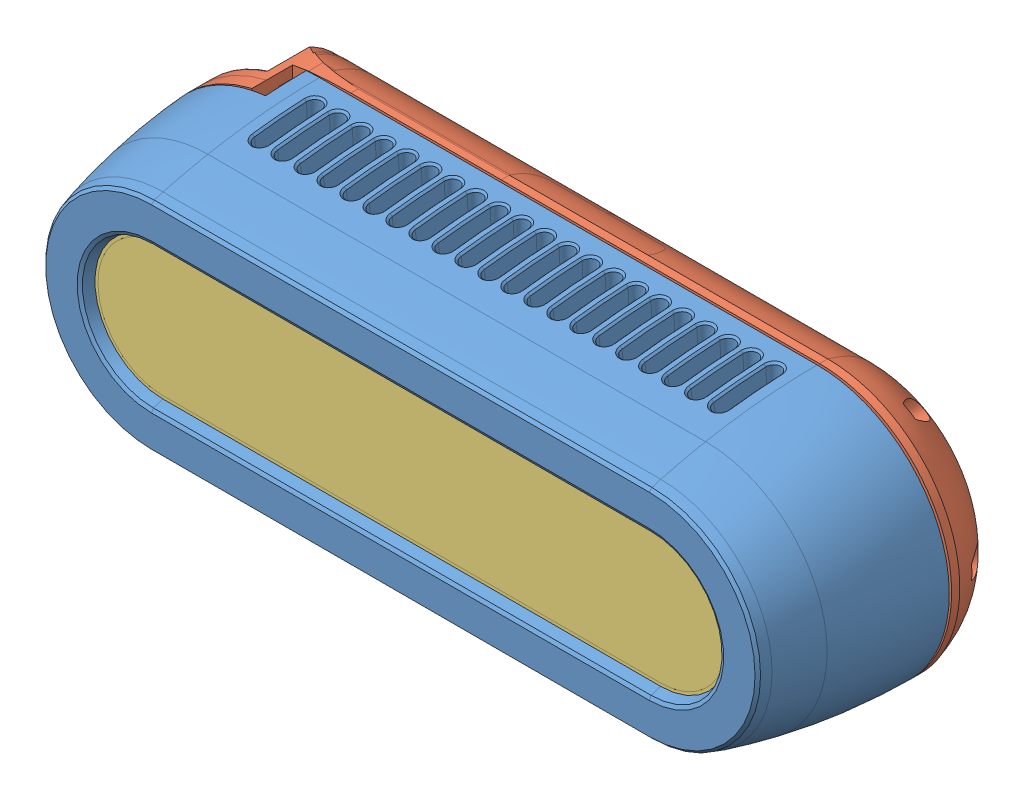
SolidWorks assembly Intel_RealSenseAssem_D435 COVER, configuration Default. Lengths in mm.
Overall size (100.25 36.56 31.79).
3 component instances, 3 part files, 5 mates.
Components (placement in the parent):
- Intel_RealSense_D435_FrontCover-1: Intel_RealSense_D435_FrontCover [Default] at origin size (99.31 34.68 21.93)
- Intel_RealSense_D435_RearCover-1: Intel_RealSense_D435_RearCover [Default] at (0 0 -0.2) size (100.25 36.56 16.67)
- IntelRealsense_D435_Multibody-1: IntelRealsense_D435_Multibody [Default] at origin size (90.13 25.18 25.29)
Mates (geometry in assembly coordinates):
- Coincident1: coincident aligned: plane of Intel_RealSense_D45_FrontCover-1 through (0 0 0) normal (0 1 0); plane of Intel_RealSense_D435_RearCover-1 through (0 0 -0.2) normal (0 1 0)
- Coincident2: coincident aligned: plane of Intel_RealSense_D45_FrontCover-1 through (0 0 0) normal (1 0 0); plane of Intel_RealSense_D435_RearCover-1 through (0 0 -0.2) normal (1 0 0)
- Distance1: distance = 0.3 mm anti-aligned: plane of Intel_RealSense_D45_FrontCover-1 through (0 0 -20.44) normal (0 0 -1); plane of Intel_RealSense_D435_RearCover-1 through (0 0 -20.74) normal (0 0 1)
- Coincident3: coordinate: point of Intel_RealSense_D435_FrontCover-1
- Coincident4: coordinate: unknown of IntelRealsense_D435_Multibody-1
